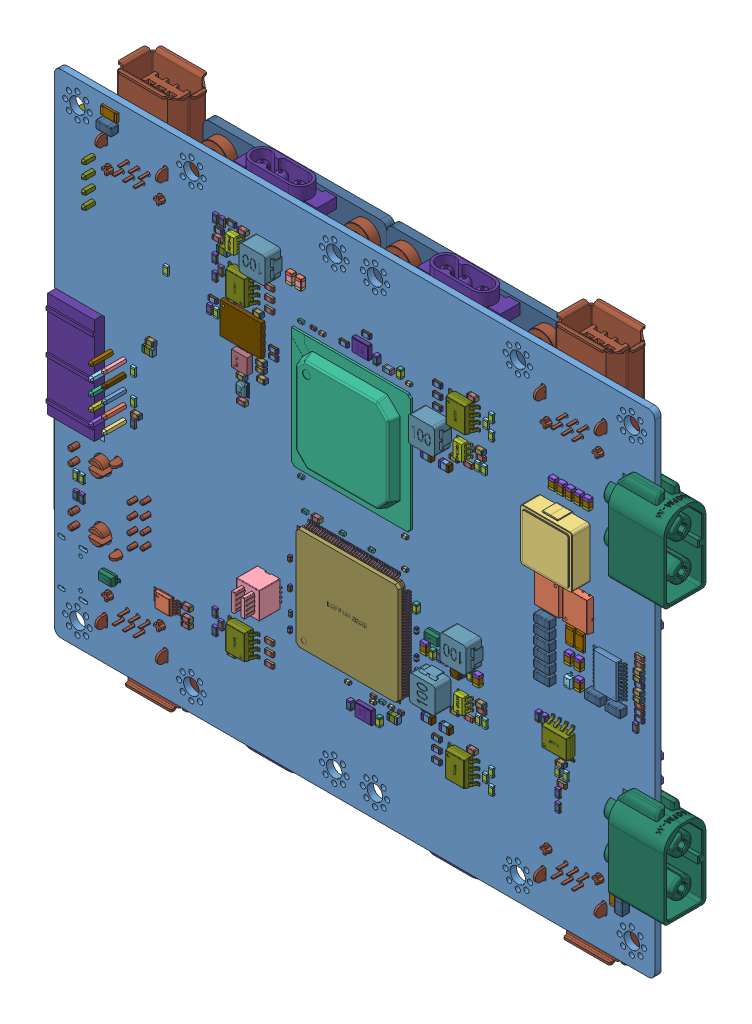
SolidWorks assembly Mother  Board, configuration 默认. Lengths in mm. (continued)
Components (placement in the parent): (continued)
- Mother  Board.step-1: Mother  Board.step [默认] at origin size (122.6 102.08 21) (continued)
  - C120.step-1: C120.step [默认] at origin size (0.8 1.6 0.8) (continued)
    - 5993853744.step-1: 5993853744.step [默认] at (62.7379 73.0251 0) x (0 1 0) z (0 0 1) size (1.6 0.8 0.8) (continued)
      - Terminal-15.step-1: Terminal-15.step [默认] at (-0.8 -0.4 0) size (1.6 0.8 0.8)
        - Open_CASCADE_STEP_translator_6.8_47.1.1-54.step-1: Open_CASCADE_STEP_translator_6.8_47.1.1-54.step [默认] at origin size (0.3 0.8 0.8)
        - Open_CASCADE_STEP_translator_6.8_47.1.2-55.step-1: Open_CASCADE_STEP_translator_6.8_47.1.2-55.step [默认] at origin size (0.3 0.8 0.8)
      - Mid_Body-6.step-1: Mid_Body-6.step [默认] at (-0.8 -0.4 0) size (1 0.8 0.8)
        - Open_CASCADE_STEP_translator_6.8_47.2.1-56.step-1: Open_CASCADE_STEP_translator_6.8_47.2.1-56.step [默认] at origin size (1 0.8 0.8)
  - C119.step-1: C119.step [默认] at origin size (1 0.5 0.5)
    - 5993845664.step-1: 5993845664.step [默认] at (58.9671 58.9279 -1.2164) x (1 0 0) z (0 0 -1) size (1 0.5 0.5)
      - Terminal-2.step-1: Terminal-2.step [默认] at (-0.5 -0.25 0) size (1 0.5 0.5)
        - Open_CASCADE_STEP_translator_6.8_54.1.1.step-1: Open_CASCADE_STEP_translator_6.8_54.1.1.step [默认] at origin size (0.25 0.5 0.5)
        - Open_CASCADE_STEP_translator_6.8_54.1.2.step-1: Open_CASCADE_STEP_translator_6.8_54.1.2.step [默认] at origin size (0.25 0.5 0.5)
      - Mid_Body-1.step-1: Mid_Body-1.step [默认] at (-0.5 -0.25 0) size (0.5 0.5 0.5)
        - Open_CASCADE_STEP_translator_6.8_54.2.1.step-1: Open_CASCADE_STEP_translator_6.8_54.2.1.step [默认] at origin size (0.5 0.5 0.5)
  - C118.step-1: C118.step [默认] at origin size (0.5 1 0.5)
    - 5993845904.step-1: 5993845904.step [默认] at (53.4671 60.4281 -1.2164) x (0 1 0) z (0 0 -1) size (1 0.5 0.5)
      - Terminal-18.step-1: Terminal-18.step [默认] at (-0.5 -0.25 0) size (1 0.5 0.5)
        - Open_CASCADE_STEP_translator_6.8_54.1.1-66.step-1: Open_CASCADE_STEP_translator_6.8_54.1.1-66.step [默认] at origin size (0.25 0.5 0.5)
        - Open_CASCADE_STEP_translator_6.8_54.1.2-67.step-1: Open_CASCADE_STEP_translator_6.8_54.1.2-67.step [默认] at origin size (0.25 0.5 0.5)
      - Mid_Body-9.step-1: Mid_Body-9.step [默认] at (-0.5 -0.25 0) size (0.5 0.5 0.5)
        - Open_CASCADE_STEP_translator_6.8_54.2.1-68.step-1: Open_CASCADE_STEP_translator_6.8_54.2.1-68.step [默认] at origin size (0.5 0.5 0.5)
  - C117.step-1: C117.step [默认] at origin size (0.5 1 0.5)
    - 5993845904.step-1: 5993845904.step [默认] at (53.4671 64.4281 -1.2164) x (0 1 0) z (0 0 -1) size (1 0.5 0.5)
      - Terminal-18.step-1: Terminal-18.step [默认] at (-0.5 -0.25 0) size (1 0.5 0.5)
        - Open_CASCADE_STEP_translator_6.8_54.1.1-66.step-1: Open_CASCADE_STEP_translator_6.8_54.1.1-66.step [默认] at origin size (0.25 0.5 0.5)
        - Open_CASCADE_STEP_translator_6.8_54.1.2-67.step-1: Open_CASCADE_STEP_translator_6.8_54.1.2-67.step [默认] at origin size (0.25 0.5 0.5)
      - Mid_Body-9.step-1: Mid_Body-9.step [默认] at (-0.5 -0.25 0) size (0.5 0.5 0.5)
        - Open_CASCADE_STEP_translator_6.8_54.2.1-68.step-1: Open_CASCADE_STEP_translator_6.8_54.2.1-68.step [默认] at origin size (0.5 0.5 0.5)
  - C115.step-1: C115.step [默认] at origin size (0.5 1 0.5)
    - 5993846064.step-1: 5993846064.step [默认] at (53.4669 62.4279 -1.2164) x (0 -1 0) z (0 0 -1) size (1 0.5 0.5)
      - Terminal-5.step-1: Terminal-5.step [默认] at (-0.5 -0.25 0) size (1 0.5 0.5)
        - Open_CASCADE_STEP_translator_6.8_54.1.1-7.step-1: Open_CASCADE_STEP_translator_6.8_54.1.1-7.step [默认] at origin size (0.25 0.5 0.5)
        - Open_CASCADE_STEP_translator_6.8_54.1.2-8.step-1: Open_CASCADE_STEP_translator_6.8_54.1.2-8.step [默认] at origin size (0.25 0.5 0.5)
      - Mid_Body-4.step-1: Mid_Body-4.step [默认] at (-0.5 -0.25 0) size (0.5 0.5 0.5)
        - Open_CASCADE_STEP_translator_6.8_54.2.1-9.step-1: Open_CASCADE_STEP_translator_6.8_54.2.1-9.step [默认] at origin size (0.5 0.5 0.5)
  - C114.step-1: C114.step [默认] at origin size (0.5 1 0.5)
    - 5993846064.step-1: 5993846064.step [默认] at (53.4669 57.4279 -1.2164) x (0 -1 0) z (0 0 -1) size (1 0.5 0.5)
      - Terminal-5.step-1: Terminal-5.step [默认] at (-0.5 -0.25 0) size (1 0.5 0.5)
        - Open_CASCADE_STEP_translator_6.8_54.1.1-7.step-1: Open_CASCADE_STEP_translator_6.8_54.1.1-7.step [默认] at origin size (0.25 0.5 0.5)
        - Open_CASCADE_STEP_translator_6.8_54.1.2-8.step-1: Open_CASCADE_STEP_translator_6.8_54.1.2-8.step [默认] at origin size (0.25 0.5 0.5)
      - Mid_Body-4.step-1: Mid_Body-4.step [默认] at (-0.5 -0.25 0) size (0.5 0.5 0.5)
        - Open_CASCADE_STEP_translator_6.8_54.2.1-9.step-1: Open_CASCADE_STEP_translator_6.8_54.2.1-9.step [默认] at origin size (0.5 0.5 0.5)
  - C113.step-1: C113.step [默认] at origin size (1 0.5 0.5)
    - 5993845664.step-1: 5993845664.step [默认] at (54.9671 58.9279 -1.2164) x (1 0 0) z (0 0 -1) size (1 0.5 0.5)
      - Terminal-2.step-1: Terminal-2.step [默认] at (-0.5 -0.25 0) size (1 0.5 0.5)
        - Open_CASCADE_STEP_translator_6.8_54.1.1.step-1: Open_CASCADE_STEP_translator_6.8_54.1.1.step [默认] at origin size (0.25 0.5 0.5)
        - Open_CASCADE_STEP_translator_6.8_54.1.2.step-1: Open_CASCADE_STEP_translator_6.8_54.1.2.step [默认] at origin size (0.25 0.5 0.5)
      - Mid_Body-1.step-1: Mid_Body-1.step [默认] at (-0.5 -0.25 0) size (0.5 0.5 0.5)
        - Open_CASCADE_STEP_translator_6.8_54.2.1.step-1: Open_CASCADE_STEP_translator_6.8_54.2.1.step [默认] at origin size (0.5 0.5 0.5)
  - C112.step-1: C112.step [默认] at origin size (1 0.5 0.5)
    - 5993845104.step-1: 5993845104.step [默认] at (56.9669 58.9281 -1.2164) x (-1 0 0) z (0 0 -1) size (1 0.5 0.5)
      - Terminal-3.step-1: Terminal-3.step [默认] at (-0.5 -0.25 0) size (1 0.5 0.5)
        - Open_CASCADE_STEP_translator_6.8_54.1.1-1.step-1: Open_CASCADE_STEP_translator_6.8_54.1.1-1.step [默认] at origin size (0.25 0.5 0.5)
        - Open_CASCADE_STEP_translator_6.8_54.1.2-2.step-1: Open_CASCADE_STEP_translator_6.8_54.1.2-2.step [默认] at origin size (0.25 0.5 0.5)
      - Mid_Body-2.step-1: Mid_Body-2.step [默认] at (-0.5 -0.25 0) size (0.5 0.5 0.5)
        - Open_CASCADE_STEP_translator_6.8_54.2.1-3.step-1: Open_CASCADE_STEP_translator_6.8_54.2.1-3.step [默认] at origin size (0.5 0.5 0.5)
  - C111.step-1: C111.step [默认] at origin size (1 0.5 0.5)
    - 5993845104.step-1: 5993845104.step [默认] at (48.9669 52.9201 -1.2164) x (-1 0 0) z (0 0 -1) size (1 0.5 0.5)
      - Terminal-3.step-1: Terminal-3.step [默认] at (-0.5 -0.25 0) size (1 0.5 0.5)
        - Open_CASCADE_STEP_translator_6.8_54.1.1-1.step-1: Open_CASCADE_STEP_translator_6.8_54.1.1-1.step [默认] at origin size (0.25 0.5 0.5)
        - Open_CASCADE_STEP_translator_6.8_54.1.2-2.step-1: Open_CASCADE_STEP_translator_6.8_54.1.2-2.step [默认] at origin size (0.25 0.5 0.5)
      - Mid_Body-2.step-1: Mid_Body-2.step [默认] at (-0.5 -0.25 0) size (0.5 0.5 0.5)
        - Open_CASCADE_STEP_translator_6.8_54.2.1-3.step-1: Open_CASCADE_STEP_translator_6.8_54.2.1-3.step [默认] at origin size (0.5 0.5 0.5)
  - C110.step-1: C110.step [默认] at origin size (1 0.5 0.5)
    - 5993845104.step-1: 5993845104.step [默认] at (47.9669 58.9281 -1.2164) x (-1 0 0) z (0 0 -1) size (1 0.5 0.5)
      - Terminal-3.step-1: Terminal-3.step [默认] at (-0.5 -0.25 0) size (1 0.5 0.5)
        - Open_CASCADE_STEP_translator_6.8_54.1.1-1.step-1: Open_CASCADE_STEP_translator_6.8_54.1.1-1.step [默认] at origin size (0.25 0.5 0.5)
        - Open_CASCADE_STEP_translator_6.8_54.1.2-2.step-1: Open_CASCADE_STEP_translator_6.8_54.1.2-2.step [默认] at origin size (0.25 0.5 0.5)
      - Mid_Body-2.step-1: Mid_Body-2.step [默认] at (-0.5 -0.25 0) size (0.5 0.5 0.5)
        - Open_CASCADE_STEP_translator_6.8_54.2.1-3.step-1: Open_CASCADE_STEP_translator_6.8_54.2.1-3.step [默认] at origin size (0.5 0.5 0.5)
  - C109.step-1: C109.step [默认] at origin size (1 0.5 0.5)
    - 5993845104.step-1: 5993845104.step [默认] at (51.9669 58.9281 -1.2164) x (-1 0 0) z (0 0 -1) size (1 0.5 0.5)
      - Terminal-3.step-1: Terminal-3.step [默认] at (-0.5 -0.25 0) size (1 0.5 0.5)
        - Open_CASCADE_STEP_translator_6.8_54.1.1-1.step-1: Open_CASCADE_STEP_translator_6.8_54.1.1-1.step [默认] at origin size (0.25 0.5 0.5)
        - Open_CASCADE_STEP_translator_6.8_54.1.2-2.step-1: Open_CASCADE_STEP_translator_6.8_54.1.2-2.step [默认] at origin size (0.25 0.5 0.5)
      - Mid_Body-2.step-1: Mid_Body-2.step [默认] at (-0.5 -0.25 0) size (0.5 0.5 0.5)
        - Open_CASCADE_STEP_translator_6.8_54.2.1-3.step-1: Open_CASCADE_STEP_translator_6.8_54.2.1-3.step [默认] at origin size (0.5 0.5 0.5)
  - C108.step-1: C108.step [默认] at origin size (0.5 1 0.5)
    - 5993846064.step-1: 5993846064.step [默认] at (53.4669 53.4279 -1.2164) x (0 -1 0) z (0 0 -1) size (1 0.5 0.5)
      - Terminal-5.step-1: Terminal-5.step [默认] at (-0.5 -0.25 0) size (1 0.5 0.5)
        - Open_CASCADE_STEP_translator_6.8_54.1.1-7.step-1: Open_CASCADE_STEP_translator_6.8_54.1.1-7.step [默认] at origin size (0.25 0.5 0.5)
        - Open_CASCADE_STEP_translator_6.8_54.1.2-8.step-1: Open_CASCADE_STEP_translator_6.8_54.1.2-8.step [默认] at origin size (0.25 0.5 0.5)
      - Mid_Body-4.step-1: Mid_Body-4.step [默认] at (-0.5 -0.25 0) size (0.5 0.5 0.5)
        - Open_CASCADE_STEP_translator_6.8_54.2.1-9.step-1: Open_CASCADE_STEP_translator_6.8_54.2.1-9.step [默认] at origin size (0.5 0.5 0.5)
  - C107.step-1: C107.step [默认] at origin size (1 0.5 0.5)
    - 5993845664.step-1: 5993845664.step [默认] at (49.9671 58.9279 -1.2164) x (1 0 0) z (0 0 -1) size (1 0.5 0.5)
      - Terminal-2.step-1: Terminal-2.step [默认] at (-0.5 -0.25 0) size (1 0.5 0.5)
        - Open_CASCADE_STEP_translator_6.8_54.1.1.step-1: Open_CASCADE_STEP_translator_6.8_54.1.1.step [默认] at origin size (0.25 0.5 0.5)
        - Open_CASCADE_STEP_translator_6.8_54.1.2.step-1: Open_CASCADE_STEP_translator_6.8_54.1.2.step [默认] at origin size (0.25 0.5 0.5)
      - Mid_Body-1.step-1: Mid_Body-1.step [默认] at (-0.5 -0.25 0) size (0.5 0.5 0.5)
        - Open_CASCADE_STEP_translator_6.8_54.2.1.step-1: Open_CASCADE_STEP_translator_6.8_54.2.1.step [默认] at origin size (0.5 0.5 0.5)
  - C106.step-1: C106.step [默认] at origin size (0.5 1 0.5)
    - 5993845904.step-1: 5993845904.step [默认] at (53.4671 55.4281 -1.2164) x (0 1 0) z (0 0 -1) size (1 0.5 0.5)
      - Terminal-18.step-1: Terminal-18.step [默认] at (-0.5 -0.25 0) size (1 0.5 0.5)
        - Open_CASCADE_STEP_translator_6.8_54.1.1-66.step-1: Open_CASCADE_STEP_translator_6.8_54.1.1-66.step [默认] at origin size (0.25 0.5 0.5)
        - Open_CASCADE_STEP_translator_6.8_54.1.2-67.step-1: Open_CASCADE_STEP_translator_6.8_54.1.2-67.step [默认] at origin size (0.25 0.5 0.5)
      - Mid_Body-9.step-1: Mid_Body-9.step [默认] at (-0.5 -0.25 0) size (0.5 0.5 0.5)
        - Open_CASCADE_STEP_translator_6.8_54.2.1-68.step-1: Open_CASCADE_STEP_translator_6.8_54.2.1-68.step [默认] at origin size (0.5 0.5 0.5)
  - C105.step-1: C105.step [默认] at origin size (1 0.5 0.5)
    - 5993845104.step-1: 5993845104.step [默认] at (50.9669 52.9201 -1.2164) x (-1 0 0) z (0 0 -1) size (1 0.5 0.5)
      - Terminal-3.step-1: Terminal-3.step [默认] at (-0.5 -0.25 0) size (1 0.5 0.5)
        - Open_CASCADE_STEP_translator_6.8_54.1.1-1.step-1: Open_CASCADE_STEP_translator_6.8_54.1.1-1.step [默认] at origin size (0.25 0.5 0.5)
        - Open_CASCADE_STEP_translator_6.8_54.1.2-2.step-1: Open_CASCADE_STEP_translator_6.8_54.1.2-2.step [默认] at origin size (0.25 0.5 0.5)
      - Mid_Body-2.step-1: Mid_Body-2.step [默认] at (-0.5 -0.25 0) size (0.5 0.5 0.5)
        - Open_CASCADE_STEP_translator_6.8_54.2.1-3.step-1: Open_CASCADE_STEP_translator_6.8_54.2.1-3.step [默认] at origin size (0.5 0.5 0.5)
  - C104.step-1: C104.step [默认] at origin size (0.5 1 0.5)
    - 5993845904.step-1: 5993845904.step [默认] at (47.4591 55.4281 -1.2164) x (0 1 0) z (0 0 -1) size (1 0.5 0.5)
      - Terminal-18.step-1: Terminal-18.step [默认] at (-0.5 -0.25 0) size (1 0.5 0.5)
        - Open_CASCADE_STEP_translator_6.8_54.1.1-66.step-1: Open_CASCADE_STEP_translator_6.8_54.1.1-66.step [默认] at origin size (0.25 0.5 0.5)
        - Open_CASCADE_STEP_translator_6.8_54.1.2-67.step-1: Open_CASCADE_STEP_translator_6.8_54.1.2-67.step [默认] at origin size (0.25 0.5 0.5)
      - Mid_Body-9.step-1: Mid_Body-9.step [默认] at (-0.5 -0.25 0) size (0.5 0.5 0.5)
        - Open_CASCADE_STEP_translator_6.8_54.2.1-68.step-1: Open_CASCADE_STEP_translator_6.8_54.2.1-68.step [默认] at origin size (0.5 0.5 0.5)
  - C103.step-1: C103.step [默认] at origin size (1.6 0.8 0.8)
    - 5993853264.step-1: 5993853264.step [默认] at (35.2959 69.2149 0) x (-1 0 0) z (0 0 1) size (1.6 0.8 0.8)
      - Terminal-6.step-1: Terminal-6.step [默认] at (-0.8 -0.4 0) size (1.6 0.8 0.8)
        - Open_CASCADE_STEP_translator_6.8_47.1.1-10.step-1: Open_CASCADE_STEP_translator_6.8_47.1.1-10.step [默认] at origin size (0.3 0.8 0.8)
        - Open_CASCADE_STEP_translator_6.8_47.1.2-11.step-1: Open_CASCADE_STEP_translator_6.8_47.1.2-11.step [默认] at origin size (0.3 0.8 0.8)
      - Mid_Body-5.step-1: Mid_Body-5.step [默认] at (-0.8 -0.4 0) size (1 0.8 0.8)
        - Open_CASCADE_STEP_translator_6.8_47.2.1-12.step-1: Open_CASCADE_STEP_translator_6.8_47.2.1-12.step [默认] at origin size (1 0.8 0.8)
  - C102.step-1: C102.step [默认] at origin size (1 0.5 0.5)
    - 5993845104.step-1: 5993845104.step [默认] at (48.9669 64.9361 -1.2164) x (-1 0 0) z (0 0 -1) size (1 0.5 0.5)
      - Terminal-3.step-1: Terminal-3.step [默认] at (-0.5 -0.25 0) size (1 0.5 0.5)
        - Open_CASCADE_STEP_translator_6.8_54.1.1-1.step-1: Open_CASCADE_STEP_translator_6.8_54.1.1-1.step [默认] at origin size (0.25 0.5 0.5)
        - Open_CASCADE_STEP_translator_6.8_54.1.2-2.step-1: Open_CASCADE_STEP_translator_6.8_54.1.2-2.step [默认] at origin size (0.25 0.5 0.5)
      - Mid_Body-2.step-1: Mid_Body-2.step [默认] at (-0.5 -0.25 0) size (0.5 0.5 0.5)
        - Open_CASCADE_STEP_translator_6.8_54.2.1-3.step-1: Open_CASCADE_STEP_translator_6.8_54.2.1-3.step [默认] at origin size (0.5 0.5 0.5)
  - C101.step-1: C101.step [默认] at origin size (0.5 1 0.5)
    - 5993845904.step-1: 5993845904.step [默认] at (59.4751 55.4281 -1.2164) x (0 1 0) z (0 0 -1) size (1 0.5 0.5)
      - Terminal-18.step-1: Terminal-18.step [默认] at (-0.5 -0.25 0) size (1 0.5 0.5)
        - Open_CASCADE_STEP_translator_6.8_54.1.1-66.step-1: Open_CASCADE_STEP_translator_6.8_54.1.1-66.step [默认] at origin size (0.25 0.5 0.5)
        - Open_CASCADE_STEP_translator_6.8_54.1.2-67.step-1: Open_CASCADE_STEP_translator_6.8_54.1.2-67.step [默认] at origin size (0.25 0.5 0.5)
      - Mid_Body-9.step-1: Mid_Body-9.step [默认] at (-0.5 -0.25 0) size (0.5 0.5 0.5)
        - Open_CASCADE_STEP_translator_6.8_54.2.1-68.step-1: Open_CASCADE_STEP_translator_6.8_54.2.1-68.step [默认] at origin size (0.5 0.5 0.5)
  - C99.step-1: C99.step [默认] at origin size (0.5 1 0.5)
    - 5993845904.step-1: 5993845904.step [默认] at (47.4591 64.4281 -1.2164) x (0 1 0) z (0 0 -1) size (1 0.5 0.5)
      - Terminal-18.step-1: Terminal-18.step [默认] at (-0.5 -0.25 0) size (1 0.5 0.5)
        - Open_CASCADE_STEP_translator_6.8_54.1.1-66.step-1: Open_CASCADE_STEP_translator_6.8_54.1.1-66.step [默认] at origin size (0.25 0.5 0.5)
        - Open_CASCADE_STEP_translator_6.8_54.1.2-67.step-1: Open_CASCADE_STEP_translator_6.8_54.1.2-67.step [默认] at origin size (0.25 0.5 0.5)
      - Mid_Body-9.step-1: Mid_Body-9.step [默认] at (-0.5 -0.25 0) size (0.5 0.5 0.5)
        - Open_CASCADE_STEP_translator_6.8_54.2.1-68.step-1: Open_CASCADE_STEP_translator_6.8_54.2.1-68.step [默认] at origin size (0.5 0.5 0.5)
  - C98.step-1: C98.step [默认] at origin size (0.5 1 0.5)
    - 5993845904.step-1: 5993845904.step [默认] at (59.4751 64.4281 -1.2164) x (0 1 0) z (0 0 -1) size (1 0.5 0.5)
      - Terminal-18.step-1: Terminal-18.step [默认] at (-0.5 -0.25 0) size (1 0.5 0.5)
        - Open_CASCADE_STEP_translator_6.8_54.1.1-66.step-1: Open_CASCADE_STEP_translator_6.8_54.1.1-66.step [默认] at origin size (0.25 0.5 0.5)
        - Open_CASCADE_STEP_translator_6.8_54.1.2-67.step-1: Open_CASCADE_STEP_translator_6.8_54.1.2-67.step [默认] at origin size (0.25 0.5 0.5)
      - Mid_Body-9.step-1: Mid_Body-9.step [默认] at (-0.5 -0.25 0) size (0.5 0.5 0.5)
        - Open_CASCADE_STEP_translator_6.8_54.2.1-68.step-1: Open_CASCADE_STEP_translator_6.8_54.2.1-68.step [默认] at origin size (0.5 0.5 0.5)
  - C97.step-1: C97.step [默认] at origin size (0.5 1 0.5)
    - 5993846064.step-1: 5993846064.step [默认] at (59.4749 60.4279 -1.2164) x (0 -1 0) z (0 0 -1) size (1 0.5 0.5)
      - Terminal-5.step-1: Terminal-5.step [默认] at (-0.5 -0.25 0) size (1 0.5 0.5)
        - Open_CASCADE_STEP_translator_6.8_54.1.1-7.step-1: Open_CASCADE_STEP_translator_6.8_54.1.1-7.step [默认] at origin size (0.25 0.5 0.5)
        - Open_CASCADE_STEP_translator_6.8_54.1.2-8.step-1: Open_CASCADE_STEP_translator_6.8_54.1.2-8.step [默认] at origin size (0.25 0.5 0.5)
      - Mid_Body-4.step-1: Mid_Body-4.step [默认] at (-0.5 -0.25 0) size (0.5 0.5 0.5)
        - Open_CASCADE_STEP_translator_6.8_54.2.1-9.step-1: Open_CASCADE_STEP_translator_6.8_54.2.1-9.step [默认] at origin size (0.5 0.5 0.5)
  - C96.step-1: C96.step [默认] at origin size (0.5 1 0.5)
    - 5993846064.step-1: 5993846064.step [默认] at (59.4749 57.4279 -1.2164) x (0 -1 0) z (0 0 -1) size (1 0.5 0.5)
      - Terminal-5.step-1: Terminal-5.step [默认] at (-0.5 -0.25 0) size (1 0.5 0.5)
        - Open_CASCADE_STEP_translator_6.8_54.1.1-7.step-1: Open_CASCADE_STEP_translator_6.8_54.1.1-7.step [默认] at origin size (0.25 0.5 0.5)
        - Open_CASCADE_STEP_translator_6.8_54.1.2-8.step-1: Open_CASCADE_STEP_translator_6.8_54.1.2-8.step [默认] at origin size (0.25 0.5 0.5)
      - Mid_Body-4.step-1: Mid_Body-4.step [默认] at (-0.5 -0.25 0) size (0.5 0.5 0.5)
        - Open_CASCADE_STEP_translator_6.8_54.2.1-9.step-1: Open_CASCADE_STEP_translator_6.8_54.2.1-9.step [默认] at origin size (0.5 0.5 0.5)
  - C95.step-1: C95.step [默认] at origin size (0.5 1 0.5)
    - 5993846064.step-1: 5993846064.step [默认] at (59.4749 62.4279 -1.2164) x (0 -1 0) z (0 0 -1) size (1 0.5 0.5)
      - Terminal-5.step-1: Terminal-5.step [默认] at (-0.5 -0.25 0) size (1 0.5 0.5)
        - Open_CASCADE_STEP_translator_6.8_54.1.1-7.step-1: Open_CASCADE_STEP_translator_6.8_54.1.1-7.step [默认] at origin size (0.25 0.5 0.5)
        - Open_CASCADE_STEP_translator_6.8_54.1.2-8.step-1: Open_CASCADE_STEP_translator_6.8_54.1.2-8.step [默认] at origin size (0.25 0.5 0.5)
      - Mid_Body-4.step-1: Mid_Body-4.step [默认] at (-0.5 -0.25 0) size (0.5 0.5 0.5)
        - Open_CASCADE_STEP_translator_6.8_54.2.1-9.step-1: Open_CASCADE_STEP_translator_6.8_54.2.1-9.step [默认] at origin size (0.5 0.5 0.5)
  - C94.step-1: C94.step [默认] at origin size (1 0.5 0.5)
    - 5993845104.step-1: 5993845104.step [默认] at (55.9669 52.9201 -1.2164) x (-1 0 0) z (0 0 -1) size (1 0.5 0.5)
      - Terminal-3.step-1: Terminal-3.step [默认] at (-0.5 -0.25 0) size (1 0.5 0.5)
        - Open_CASCADE_STEP_translator_6.8_54.1.1-1.step-1: Open_CASCADE_STEP_translator_6.8_54.1.1-1.step [默认] at origin size (0.25 0.5 0.5)
        - Open_CASCADE_STEP_translator_6.8_54.1.2-2.step-1: Open_CASCADE_STEP_translator_6.8_54.1.2-2.step [默认] at origin size (0.25 0.5 0.5)
      - Mid_Body-2.step-1: Mid_Body-2.step [默认] at (-0.5 -0.25 0) size (0.5 0.5 0.5)
        - Open_CASCADE_STEP_translator_6.8_54.2.1-3.step-1: Open_CASCADE_STEP_translator_6.8_54.2.1-3.step [默认] at origin size (0.5 0.5 0.5)
  - C93.step-1: C93.step [默认] at origin size (1 0.5 0.5)
    - 5993845664.step-1: 5993845664.step [默认] at (57.9671 52.9199 -1.2164) x (1 0 0) z (0 0 -1) size (1 0.5 0.5)
      - Terminal-2.step-1: Terminal-2.step [默认] at (-0.5 -0.25 0) size (1 0.5 0.5)
        - Open_CASCADE_STEP_translator_6.8_54.1.1.step-1: Open_CASCADE_STEP_translator_6.8_54.1.1.step [默认] at origin size (0.25 0.5 0.5)
        - Open_CASCADE_STEP_translator_6.8_54.1.2.step-1: Open_CASCADE_STEP_translator_6.8_54.1.2.step [默认] at origin size (0.25 0.5 0.5)
      - Mid_Body-1.step-1: Mid_Body-1.step [默认] at (-0.5 -0.25 0) size (0.5 0.5 0.5)
        - Open_CASCADE_STEP_translator_6.8_54.2.1.step-1: Open_CASCADE_STEP_translator_6.8_54.2.1.step [默认] at origin size (0.5 0.5 0.5)
  - C92.step-1: C92.step [默认] at origin size (1 0.5 0.5)
    - 5993845664.step-1: 5993845664.step [默认] at (50.9671 64.9359 -1.2164) x (1 0 0) z (0 0 -1) size (1 0.5 0.5)
      - Terminal-2.step-1: Terminal-2.step [默认] at (-0.5 -0.25 0) size (1 0.5 0.5)
        - Open_CASCADE_STEP_translator_6.8_54.1.1.step-1: Open_CASCADE_STEP_translator_6.8_54.1.1.step [默认] at origin size (0.25 0.5 0.5)
        - Open_CASCADE_STEP_translator_6.8_54.1.2.step-1: Open_CASCADE_STEP_translator_6.8_54.1.2.step [默认] at origin size (0.25 0.5 0.5)
      - Mid_Body-1.step-1: Mid_Body-1.step [默认] at (-0.5 -0.25 0) size (0.5 0.5 0.5)
        - Open_CASCADE_STEP_translator_6.8_54.2.1.step-1: Open_CASCADE_STEP_translator_6.8_54.2.1.step [默认] at origin size (0.5 0.5 0.5)
  - C91.step-1: C91.step [默认] at origin size (0.5 1 0.5)
    - 5993846064.step-1: 5993846064.step [默认] at (47.4589 57.4279 -1.2164) x (0 -1 0) z (0 0 -1) size (1 0.5 0.5)
      - Terminal-5.step-1: Terminal-5.step [默认] at (-0.5 -0.25 0) size (1 0.5 0.5)
        - Open_CASCADE_STEP_translator_6.8_54.1.1-7.step-1: Open_CASCADE_STEP_translator_6.8_54.1.1-7.step [默认] at origin size (0.25 0.5 0.5)
        - Open_CASCADE_STEP_translator_6.8_54.1.2-8.step-1: Open_CASCADE_STEP_translator_6.8_54.1.2-8.step [默认] at origin size (0.25 0.5 0.5)
      - Mid_Body-4.step-1: Mid_Body-4.step [默认] at (-0.5 -0.25 0) size (0.5 0.5 0.5)
        - Open_CASCADE_STEP_translator_6.8_54.2.1-9.step-1: Open_CASCADE_STEP_translator_6.8_54.2.1-9.step [默认] at origin size (0.5 0.5 0.5)
  - C89.step-1: C89.step [默认] at origin size (0.5 1 0.5)
    - 5993846064.step-1: 5993846064.step [默认] at (59.4749 53.4279 -1.2164) x (0 -1 0) z (0 0 -1) size (1 0.5 0.5)
      - Terminal-5.step-1: Terminal-5.step [默认] at (-0.5 -0.25 0) size (1 0.5 0.5)
        - Open_CASCADE_STEP_translator_6.8_54.1.1-7.step-1: Open_CASCADE_STEP_translator_6.8_54.1.1-7.step [默认] at origin size (0.25 0.5 0.5)
        - Open_CASCADE_STEP_translator_6.8_54.1.2-8.step-1: Open_CASCADE_STEP_translator_6.8_54.1.2-8.step [默认] at origin size (0.25 0.5 0.5)
      - Mid_Body-4.step-1: Mid_Body-4.step [默认] at (-0.5 -0.25 0) size (0.5 0.5 0.5)
        - Open_CASCADE_STEP_translator_6.8_54.2.1-9.step-1: Open_CASCADE_STEP_translator_6.8_54.2.1-9.step [默认] at origin size (0.5 0.5 0.5)
  - C88.step-1: C88.step [默认] at origin size (1 0.5 0.5)
    - 5993845664.step-1: 5993845664.step [默认] at (57.9671 64.9359 -1.2164) x (1 0 0) z (0 0 -1) size (1 0.5 0.5)
      - Terminal-2.step-1: Terminal-2.step [默认] at (-0.5 -0.25 0) size (1 0.5 0.5)
        - Open_CASCADE_STEP_translator_6.8_54.1.1.step-1: Open_CASCADE_STEP_translator_6.8_54.1.1.step [默认] at origin size (0.25 0.5 0.5)
        - Open_CASCADE_STEP_translator_6.8_54.1.2.step-1: Open_CASCADE_STEP_translator_6.8_54.1.2.step [默认] at origin size (0.25 0.5 0.5)
      - Mid_Body-1.step-1: Mid_Body-1.step [默认] at (-0.5 -0.25 0) size (0.5 0.5 0.5)
        - Open_CASCADE_STEP_translator_6.8_54.2.1.step-1: Open_CASCADE_STEP_translator_6.8_54.2.1.step [默认] at origin size (0.5 0.5 0.5)
  - C87.step-1: C87.step [默认] at origin size (0.5 1 0.5)
    - 5993846064.step-1: 5993846064.step [默认] at (47.4589 62.4279 -1.2164) x (0 -1 0) z (0 0 -1) size (1 0.5 0.5)
      - Terminal-5.step-1: Terminal-5.step [默认] at (-0.5 -0.25 0) size (1 0.5 0.5)
        - Open_CASCADE_STEP_translator_6.8_54.1.1-7.step-1: Open_CASCADE_STEP_translator_6.8_54.1.1-7.step [默认] at origin size (0.25 0.5 0.5)
        - Open_CASCADE_STEP_translator_6.8_54.1.2-8.step-1: Open_CASCADE_STEP_translator_6.8_54.1.2-8.step [默认] at origin size (0.25 0.5 0.5)
      - Mid_Body-4.step-1: Mid_Body-4.step [默认] at (-0.5 -0.25 0) size (0.5 0.5 0.5)
        - Open_CASCADE_STEP_translator_6.8_54.2.1-9.step-1: Open_CASCADE_STEP_translator_6.8_54.2.1-9.step [默认] at origin size (0.5 0.5 0.5)
  - C86.step-1: C86.step [默认] at origin size (1.6 0.8 0.8)
    - 5993853264.step-1: 5993853264.step [默认] at (11.8109 40.5129 0) x (-1 0 0) z (0 0 1) size (1.6 0.8 0.8)
      - Terminal-6.step-1: Terminal-6.step [默认] at (-0.8 -0.4 0) size (1.6 0.8 0.8)
        - Open_CASCADE_STEP_translator_6.8_47.1.1-10.step-1: Open_CASCADE_STEP_translator_6.8_47.1.1-10.step [默认] at origin size (0.3 0.8 0.8)
        - Open_CASCADE_STEP_translator_6.8_47.1.2-11.step-1: Open_CASCADE_STEP_translator_6.8_47.1.2-11.step [默认] at origin size (0.3 0.8 0.8)
      - Mid_Body-5.step-1: Mid_Body-5.step [默认] at (-0.8 -0.4 0) size (1 0.8 0.8)
        - Open_CASCADE_STEP_translator_6.8_47.2.1-12.step-1: Open_CASCADE_STEP_translator_6.8_47.2.1-12.step [默认] at origin size (1 0.8 0.8)
  - C85.step-1: C85.step [默认] at origin size (1 0.5 0.5)
    - 5993845104.step-1: 5993845104.step [默认] at (52.9669 51.9281 -1.2164) x (-1 0 0) z (0 0 -1) size (1 0.5 0.5)
      - Terminal-3.step-1: Terminal-3.step [默认] at (-0.5 -0.25 0) size (1 0.5 0.5)
        - Open_CASCADE_STEP_translator_6.8_54.1.1-1.step-1: Open_CASCADE_STEP_translator_6.8_54.1.1-1.step [默认] at origin size (0.25 0.5 0.5)
        - Open_CASCADE_STEP_translator_6.8_54.1.2-2.step-1: Open_CASCADE_STEP_translator_6.8_54.1.2-2.step [默认] at origin size (0.25 0.5 0.5)
      - Mid_Body-2.step-1: Mid_Body-2.step [默认] at (-0.5 -0.25 0) size (0.5 0.5 0.5)
        - Open_CASCADE_STEP_translator_6.8_54.2.1-3.step-1: Open_CASCADE_STEP_translator_6.8_54.2.1-3.step [默认] at origin size (0.5 0.5 0.5)
  - C84.step-1: C84.step [默认] at origin size (1 0.5 0.5)
    - 5993845104.step-1: 5993845104.step [默认] at (61.9669 64.9361 -1.2164) x (-1 0 0) z (0 0 -1) size (1 0.5 0.5)
      - Terminal-3.step-1: Terminal-3.step [默认] at (-0.5 -0.25 0) size (1 0.5 0.5)
        - Open_CASCADE_STEP_translator_6.8_54.1.1-1.step-1: Open_CASCADE_STEP_translator_6.8_54.1.1-1.step [默认] at origin size (0.25 0.5 0.5)
        - Open_CASCADE_STEP_translator_6.8_54.1.2-2.step-1: Open_CASCADE_STEP_translator_6.8_54.1.2-2.step [默认] at origin size (0.25 0.5 0.5)
      - Mid_Body-2.step-1: Mid_Body-2.step [默认] at (-0.5 -0.25 0) size (0.5 0.5 0.5)
        - Open_CASCADE_STEP_translator_6.8_54.2.1-3.step-1: Open_CASCADE_STEP_translator_6.8_54.2.1-3.step [默认] at origin size (0.5 0.5 0.5)
  - C83.step-1: C83.step [默认] at origin size (1 0.5 0.5)
    - 5993845104.step-1: 5993845104.step [默认] at (50.9669 51.9281 -1.2164) x (-1 0 0) z (0 0 -1) size (1 0.5 0.5)
      - Terminal-3.step-1: Terminal-3.step [默认] at (-0.5 -0.25 0) size (1 0.5 0.5)
        - Open_CASCADE_STEP_translator_6.8_54.1.1-1.step-1: Open_CASCADE_STEP_translator_6.8_54.1.1-1.step [默认] at origin size (0.25 0.5 0.5)
        - Open_CASCADE_STEP_translator_6.8_54.1.2-2.step-1: Open_CASCADE_STEP_translator_6.8_54.1.2-2.step [默认] at origin size (0.25 0.5 0.5)
      - Mid_Body-2.step-1: Mid_Body-2.step [默认] at (-0.5 -0.25 0) size (0.5 0.5 0.5)
        - Open_CASCADE_STEP_translator_6.8_54.2.1-3.step-1: Open_CASCADE_STEP_translator_6.8_54.2.1-3.step [默认] at origin size (0.5 0.5 0.5)
  - C81.step-1: C81.step [默认] at origin size (0.5 1 0.5)
    - 5993845904.step-1: 5993845904.step [默认] at (47.4671 50.4281 -1.2164) x (0 1 0) z (0 0 -1) size (1 0.5 0.5)
      - Terminal-18.step-1: Terminal-18.step [默认] at (-0.5 -0.25 0) size (1 0.5 0.5)
        - Open_CASCADE_STEP_translator_6.8_54.1.1-66.step-1: Open_CASCADE_STEP_translator_6.8_54.1.1-66.step [默认] at origin size (0.25 0.5 0.5)
        - Open_CASCADE_STEP_translator_6.8_54.1.2-67.step-1: Open_CASCADE_STEP_translator_6.8_54.1.2-67.step [默认] at origin size (0.25 0.5 0.5)
      - Mid_Body-9.step-1: Mid_Body-9.step [默认] at (-0.5 -0.25 0) size (0.5 0.5 0.5)
        - Open_CASCADE_STEP_translator_6.8_54.2.1-68.step-1: Open_CASCADE_STEP_translator_6.8_54.2.1-68.step [默认] at origin size (0.5 0.5 0.5)
  - C80.step-1: C80.step [默认] at origin size (1 0.5 0.5)
    - 5993845664.step-1: 5993845664.step [默认] at (59.9671 51.9279 -1.2164) x (1 0 0) z (0 0 -1) size (1 0.5 0.5)
      - Terminal-2.step-1: Terminal-2.step [默认] at (-0.5 -0.25 0) size (1 0.5 0.5)
        - Open_CASCADE_STEP_translator_6.8_54.1.1.step-1: Open_CASCADE_STEP_translator_6.8_54.1.1.step [默认] at origin size (0.25 0.5 0.5)
        - Open_CASCADE_STEP_translator_6.8_54.1.2.step-1: Open_CASCADE_STEP_translator_6.8_54.1.2.step [默认] at origin size (0.25 0.5 0.5)
      - Mid_Body-1.step-1: Mid_Body-1.step [默认] at (-0.5 -0.25 0) size (0.5 0.5 0.5)
        - Open_CASCADE_STEP_translator_6.8_54.2.1.step-1: Open_CASCADE_STEP_translator_6.8_54.2.1.step [默认] at origin size (0.5 0.5 0.5)
  - C79.step-1: C79.step [默认] at origin size (1 0.5 0.5)
    - 5993845104.step-1: 5993845104.step [默认] at (61.9669 62.9361 -1.2164) x (-1 0 0) z (0 0 -1) size (1 0.5 0.5)
      - Terminal-3.step-1: Terminal-3.step [默认] at (-0.5 -0.25 0) size (1 0.5 0.5)
        - Open_CASCADE_STEP_translator_6.8_54.1.1-1.step-1: Open_CASCADE_STEP_translator_6.8_54.1.1-1.step [默认] at origin size (0.25 0.5 0.5)
        - Open_CASCADE_STEP_translator_6.8_54.1.2-2.step-1: Open_CASCADE_STEP_translator_6.8_54.1.2-2.step [默认] at origin size (0.25 0.5 0.5)
      - Mid_Body-2.step-1: Mid_Body-2.step [默认] at (-0.5 -0.25 0) size (0.5 0.5 0.5)
        - Open_CASCADE_STEP_translator_6.8_54.2.1-3.step-1: Open_CASCADE_STEP_translator_6.8_54.2.1-3.step [默认] at origin size (0.5 0.5 0.5)
  - C78.step-1: C78.step [默认] at origin size (1 0.5 0.5)
    - 5993845104.step-1: 5993845104.step [默认] at (61.9669 52.9201 -1.2164) x (-1 0 0) z (0 0 -1) size (1 0.5 0.5)
      - Terminal-3.step-1: Terminal-3.step [默认] at (-0.5 -0.25 0) size (1 0.5 0.5)
        - Open_CASCADE_STEP_translator_6.8_54.1.1-1.step-1: Open_CASCADE_STEP_translator_6.8_54.1.1-1.step [默认] at origin size (0.25 0.5 0.5)
        - Open_CASCADE_STEP_translator_6.8_54.1.2-2.step-1: Open_CASCADE_STEP_translator_6.8_54.1.2-2.step [默认] at origin size (0.25 0.5 0.5)
      - Mid_Body-2.step-1: Mid_Body-2.step [默认] at (-0.5 -0.25 0) size (0.5 0.5 0.5)
        - Open_CASCADE_STEP_translator_6.8_54.2.1-3.step-1: Open_CASCADE_STEP_translator_6.8_54.2.1-3.step [默认] at origin size (0.5 0.5 0.5)
  - C77.step-1: C77.step [默认] at origin size (1 0.5 0.5)
    - 5993845104.step-1: 5993845104.step [默认] at (61.9669 50.9281 -1.2164) x (-1 0 0) z (0 0 -1) size (1 0.5 0.5)
      - Terminal-3.step-1: Terminal-3.step [默认] at (-0.5 -0.25 0) size (1 0.5 0.5)
        - Open_CASCADE_STEP_translator_6.8_54.1.1-1.step-1: Open_CASCADE_STEP_translator_6.8_54.1.1-1.step [默认] at origin size (0.25 0.5 0.5)
        - Open_CASCADE_STEP_translator_6.8_54.1.2-2.step-1: Open_CASCADE_STEP_translator_6.8_54.1.2-2.step [默认] at origin size (0.25 0.5 0.5)
      - Mid_Body-2.step-1: Mid_Body-2.step [默认] at (-0.5 -0.25 0) size (0.5 0.5 0.5)
        - Open_CASCADE_STEP_translator_6.8_54.2.1-3.step-1: Open_CASCADE_STEP_translator_6.8_54.2.1-3.step [默认] at origin size (0.5 0.5 0.5)
  - C76.step-1: C76.step [默认] at origin size (1 0.5 0.5)
    - 5993845104.step-1: 5993845104.step [默认] at (61.9669 58.9281 -1.2164) x (-1 0 0) z (0 0 -1) size (1 0.5 0.5)
      - Terminal-3.step-1: Terminal-3.step [默认] at (-0.5 -0.25 0) size (1 0.5 0.5)
        - Open_CASCADE_STEP_translator_6.8_54.1.1-1.step-1: Open_CASCADE_STEP_translator_6.8_54.1.1-1.step [默认] at origin size (0.25 0.5 0.5)
        - Open_CASCADE_STEP_translator_6.8_54.1.2-2.step-1: Open_CASCADE_STEP_translator_6.8_54.1.2-2.step [默认] at origin size (0.25 0.5 0.5)
      - Mid_Body-2.step-1: Mid_Body-2.step [默认] at (-0.5 -0.25 0) size (0.5 0.5 0.5)
        - Open_CASCADE_STEP_translator_6.8_54.2.1-3.step-1: Open_CASCADE_STEP_translator_6.8_54.2.1-3.step [默认] at origin size (0.5 0.5 0.5)
  - C75.step-1: C75.step [默认] at origin size (0.5 1 0.5)
    - 5993846064.step-1: 5993846064.step [默认] at (53.4669 67.4279 -1.2164) x (0 -1 0) z (0 0 -1) size (1 0.5 0.5)
      - Terminal-5.step-1: Terminal-5.step [默认] at (-0.5 -0.25 0) size (1 0.5 0.5)
        - Open_CASCADE_STEP_translator_6.8_54.1.1-7.step-1: Open_CASCADE_STEP_translator_6.8_54.1.1-7.step [默认] at origin size (0.25 0.5 0.5)
        - Open_CASCADE_STEP_translator_6.8_54.1.2-8.step-1: Open_CASCADE_STEP_translator_6.8_54.1.2-8.step [默认] at origin size (0.25 0.5 0.5)
      - Mid_Body-4.step-1: Mid_Body-4.step [默认] at (-0.5 -0.25 0) size (0.5 0.5 0.5)
        - Open_CASCADE_STEP_translator_6.8_54.2.1-9.step-1: Open_CASCADE_STEP_translator_6.8_54.2.1-9.step [默认] at origin size (0.5 0.5 0.5)
  - C74.step-1: C74.step [默认] at origin size (1 0.5 0.5)
    - 5993845664.step-1: 5993845664.step [默认] at (44.9671 57.9279 -1.2164) x (1 0 0) z (0 0 -1) size (1 0.5 0.5)
      - Terminal-2.step-1: Terminal-2.step [默认] at (-0.5 -0.25 0) size (1 0.5 0.5)
        - Open_CASCADE_STEP_translator_6.8_54.1.1.step-1: Open_CASCADE_STEP_translator_6.8_54.1.1.step [默认] at origin size (0.25 0.5 0.5)
        - Open_CASCADE_STEP_translator_6.8_54.1.2.step-1: Open_CASCADE_STEP_translator_6.8_54.1.2.step [默认] at origin size (0.25 0.5 0.5)
      - Mid_Body-1.step-1: Mid_Body-1.step [默认] at (-0.5 -0.25 0) size (0.5 0.5 0.5)
        - Open_CASCADE_STEP_translator_6.8_54.2.1.step-1: Open_CASCADE_STEP_translator_6.8_54.2.1.step [默认] at origin size (0.5 0.5 0.5)
  - C73.step-1: C73.step [默认] at origin size (0.5 1 0.5)
    - 5993846064.step-1: 5993846064.step [默认] at (57.4589 67.4279 -1.2164) x (0 -1 0) z (0 0 -1) size (1 0.5 0.5)
      - Terminal-5.step-1: Terminal-5.step [默认] at (-0.5 -0.25 0) size (1 0.5 0.5)
        - Open_CASCADE_STEP_translator_6.8_54.1.1-7.step-1: Open_CASCADE_STEP_translator_6.8_54.1.1-7.step [默认] at origin size (0.25 0.5 0.5)
        - Open_CASCADE_STEP_translator_6.8_54.1.2-8.step-1: Open_CASCADE_STEP_translator_6.8_54.1.2-8.step [默认] at origin size (0.25 0.5 0.5)
      - Mid_Body-4.step-1: Mid_Body-4.step [默认] at (-0.5 -0.25 0) size (0.5 0.5 0.5)
        - Open_CASCADE_STEP_translator_6.8_54.2.1-9.step-1: Open_CASCADE_STEP_translator_6.8_54.2.1-9.step [默认] at origin size (0.5 0.5 0.5)
  - C69.step-1: C69.step [默认] at origin size (0.5 1 0.5)
    - 5993846064.step-1: 5993846064.step [默认] at (51.4669 67.4279 -1.2164) x (0 -1 0) z (0 0 -1) size (1 0.5 0.5)
      - Terminal-5.step-1: Terminal-5.step [默认] at (-0.5 -0.25 0) size (1 0.5 0.5)
        - Open_CASCADE_STEP_translator_6.8_54.1.1-7.step-1: Open_CASCADE_STEP_translator_6.8_54.1.1-7.step [默认] at origin size (0.25 0.5 0.5)
        - Open_CASCADE_STEP_translator_6.8_54.1.2-8.step-1: Open_CASCADE_STEP_translator_6.8_54.1.2-8.step [默认] at origin size (0.25 0.5 0.5)
      - Mid_Body-4.step-1: Mid_Body-4.step [默认] at (-0.5 -0.25 0) size (0.5 0.5 0.5)
        - Open_CASCADE_STEP_translator_6.8_54.2.1-9.step-1: Open_CASCADE_STEP_translator_6.8_54.2.1-9.step [默认] at origin size (0.5 0.5 0.5)
  - C68.step-1: C68.step [默认] at origin size (1 0.5 0.5)
    - 5993845664.step-1: 5993845664.step [默认] at (54.9671 51.9279 -1.2164) x (1 0 0) z (0 0 -1) size (1 0.5 0.5)
      - Terminal-2.step-1: Terminal-2.step [默认] at (-0.5 -0.25 0) size (1 0.5 0.5)
        - Open_CASCADE_STEP_translator_6.8_54.1.1.step-1: Open_CASCADE_STEP_translator_6.8_54.1.1.step [默认] at origin size (0.25 0.5 0.5)
        - Open_CASCADE_STEP_translator_6.8_54.1.2.step-1: Open_CASCADE_STEP_translator_6.8_54.1.2.step [默认] at origin size (0.25 0.5 0.5)
      - Mid_Body-1.step-1: Mid_Body-1.step [默认] at (-0.5 -0.25 0) size (0.5 0.5 0.5)
        - Open_CASCADE_STEP_translator_6.8_54.2.1.step-1: Open_CASCADE_STEP_translator_6.8_54.2.1.step [默认] at origin size (0.5 0.5 0.5)
  - C67.step-1: C67.step [默认] at origin size (0.5 1 0.5)
    - 5993846064.step-1: 5993846064.step [默认] at (55.4589 67.4279 -1.2164) x (0 -1 0) z (0 0 -1) size (1 0.5 0.5)
      - Terminal-5.step-1: Terminal-5.step [默认] at (-0.5 -0.25 0) size (1 0.5 0.5)
        - Open_CASCADE_STEP_translator_6.8_54.1.1-7.step-1: Open_CASCADE_STEP_translator_6.8_54.1.1-7.step [默认] at origin size (0.25 0.5 0.5)
        - Open_CASCADE_STEP_translator_6.8_54.1.2-8.step-1: Open_CASCADE_STEP_translator_6.8_54.1.2-8.step [默认] at origin size (0.25 0.5 0.5)
      - Mid_Body-4.step-1: Mid_Body-4.step [默认] at (-0.5 -0.25 0) size (0.5 0.5 0.5)
        - Open_CASCADE_STEP_translator_6.8_54.2.1-9.step-1: Open_CASCADE_STEP_translator_6.8_54.2.1-9.step [默认] at origin size (0.5 0.5 0.5)
  - C66.step-1: C66.step [默认] at origin size (1 0.5 0.5)
    - 5993845664.step-1: 5993845664.step [默认] at (44.9671 61.9199 -1.2164) x (1 0 0) z (0 0 -1) size (1 0.5 0.5)
      - Terminal-2.step-1: Terminal-2.step [默认] at (-0.5 -0.25 0) size (1 0.5 0.5)
        - Open_CASCADE_STEP_translator_6.8_54.1.1.step-1: Open_CASCADE_STEP_translator_6.8_54.1.1.step [默认] at origin size (0.25 0.5 0.5)
        - Open_CASCADE_STEP_translator_6.8_54.1.2.step-1: Open_CASCADE_STEP_translator_6.8_54.1.2.step [默认] at origin size (0.25 0.5 0.5)
      - Mid_Body-1.step-1: Mid_Body-1.step [默认] at (-0.5 -0.25 0) size (0.5 0.5 0.5)
        - Open_CASCADE_STEP_translator_6.8_54.2.1.step-1: Open_CASCADE_STEP_translator_6.8_54.2.1.step [默认] at origin size (0.5 0.5 0.5)
  - C65.step-1: C65.step [默认] at origin size (0.5 1 0.5)
    - 5993846064.step-1: 5993846064.step [默认] at (59.4749 67.4279 -1.2164) x (0 -1 0) z (0 0 -1) size (1 0.5 0.5)
      - Terminal-5.step-1: Terminal-5.step [默认] at (-0.5 -0.25 0) size (1 0.5 0.5)
        - Open_CASCADE_STEP_translator_6.8_54.1.1-7.step-1: Open_CASCADE_STEP_translator_6.8_54.1.1-7.step [默认] at origin size (0.25 0.5 0.5)
        - Open_CASCADE_STEP_translator_6.8_54.1.2-8.step-1: Open_CASCADE_STEP_translator_6.8_54.1.2-8.step [默认] at origin size (0.25 0.5 0.5)
      - Mid_Body-4.step-1: Mid_Body-4.step [默认] at (-0.5 -0.25 0) size (0.5 0.5 0.5)
        - Open_CASCADE_STEP_translator_6.8_54.2.1-9.step-1: Open_CASCADE_STEP_translator_6.8_54.2.1-9.step [默认] at origin size (0.5 0.5 0.5)
  - C63.step-1: C63.step [默认] at origin size (1 0.5 0.5)
    - 5993845664.step-1: 5993845664.step [默认] at (44.9671 63.9279 -1.2164) x (1 0 0) z (0 0 -1) size (1 0.5 0.5)
      - Terminal-2.step-1: Terminal-2.step [默认] at (-0.5 -0.25 0) size (1 0.5 0.5)
        - Open_CASCADE_STEP_translator_6.8_54.1.1.step-1: Open_CASCADE_STEP_translator_6.8_54.1.1.step [默认] at origin size (0.25 0.5 0.5)
        - Open_CASCADE_STEP_translator_6.8_54.1.2.step-1: Open_CASCADE_STEP_translator_6.8_54.1.2.step [默认] at origin size (0.25 0.5 0.5)
      - Mid_Body-1.step-1: Mid_Body-1.step [默认] at (-0.5 -0.25 0) size (0.5 0.5 0.5)
        - Open_CASCADE_STEP_translator_6.8_54.2.1.step-1: Open_CASCADE_STEP_translator_6.8_54.2.1.step [默认] at origin size (0.5 0.5 0.5)
  - C62.step-1: C62.step [默认] at origin size (0.5 1 0.5)
    - 5993846064.step-1: 5993846064.step [默认] at (47.4589 67.4279 -1.2164) x (0 -1 0) z (0 0 -1) size (1 0.5 0.5)
      - Terminal-5.step-1: Terminal-5.step [默认] at (-0.5 -0.25 0) size (1 0.5 0.5)
        - Open_CASCADE_STEP_translator_6.8_54.1.1-7.step-1: Open_CASCADE_STEP_translator_6.8_54.1.1-7.step [默认] at origin size (0.25 0.5 0.5)
        - Open_CASCADE_STEP_translator_6.8_54.1.2-8.step-1: Open_CASCADE_STEP_translator_6.8_54.1.2-8.step [默认] at origin size (0.25 0.5 0.5)
      - Mid_Body-4.step-1: Mid_Body-4.step [默认] at (-0.5 -0.25 0) size (0.5 0.5 0.5)
        - Open_CASCADE_STEP_translator_6.8_54.2.1-9.step-1: Open_CASCADE_STEP_translator_6.8_54.2.1-9.step [默认] at origin size (0.5 0.5 0.5)
  - C61.step-1: C61.step [默认] at origin size (1 0.5 0.5)
    - 5993845664.step-1: 5993845664.step [默认] at (44.9671 51.9279 -1.2164) x (1 0 0) z (0 0 -1) size (1 0.5 0.5)
      - Terminal-2.step-1: Terminal-2.step [默认] at (-0.5 -0.25 0) size (1 0.5 0.5)
        - Open_CASCADE_STEP_translator_6.8_54.1.1.step-1: Open_CASCADE_STEP_translator_6.8_54.1.1.step [默认] at origin size (0.25 0.5 0.5)
        - Open_CASCADE_STEP_translator_6.8_54.1.2.step-1: Open_CASCADE_STEP_translator_6.8_54.1.2.step [默认] at origin size (0.25 0.5 0.5)
      - Mid_Body-1.step-1: Mid_Body-1.step [默认] at (-0.5 -0.25 0) size (0.5 0.5 0.5)
        - Open_CASCADE_STEP_translator_6.8_54.2.1.step-1: Open_CASCADE_STEP_translator_6.8_54.2.1.step [默认] at origin size (0.5 0.5 0.5)
  - C60.step-1: C60.step [默认] at origin size (1 0.5 0.5)
    - 5993845664.step-1: 5993845664.step [默认] at (44.9671 65.9279 -1.2164) x (1 0 0) z (0 0 -1) size (1 0.5 0.5)
      - Terminal-2.step-1: Terminal-2.step [默认] at (-0.5 -0.25 0) size (1 0.5 0.5)
        - Open_CASCADE_STEP_translator_6.8_54.1.1.step-1: Open_CASCADE_STEP_translator_6.8_54.1.1.step [默认] at origin size (0.25 0.5 0.5)
        - Open_CASCADE_STEP_translator_6.8_54.1.2.step-1: Open_CASCADE_STEP_translator_6.8_54.1.2.step [默认] at origin size (0.25 0.5 0.5)
      - Mid_Body-1.step-1: Mid_Body-1.step [默认] at (-0.5 -0.25 0) size (0.5 0.5 0.5)
        - Open_CASCADE_STEP_translator_6.8_54.2.1.step-1: Open_CASCADE_STEP_translator_6.8_54.2.1.step [默认] at origin size (0.5 0.5 0.5)
  - C59.step-1: C59.step [默认] at origin size (1 0.5 0.5)
    - 5993845664.step-1: 5993845664.step [默认] at (44.9671 49.9199 -1.2164) x (1 0 0) z (0 0 -1) size (1 0.5 0.5)
      - Terminal-2.step-1: Terminal-2.step [默认] at (-0.5 -0.25 0) size (1 0.5 0.5)
        - Open_CASCADE_STEP_translator_6.8_54.1.1.step-1: Open_CASCADE_STEP_translator_6.8_54.1.1.step [默认] at origin size (0.25 0.5 0.5)
        - Open_CASCADE_STEP_translator_6.8_54.1.2.step-1: Open_CASCADE_STEP_translator_6.8_54.1.2.step [默认] at origin size (0.25 0.5 0.5)
      - Mid_Body-1.step-1: Mid_Body-1.step [默认] at (-0.5 -0.25 0) size (0.5 0.5 0.5)
        - Open_CASCADE_STEP_translator_6.8_54.2.1.step-1: Open_CASCADE_STEP_translator_6.8_54.2.1.step [默认] at origin size (0.5 0.5 0.5)
  - C58.step-1: C58.step [默认] at origin size (1 0.5 0.5)
    - 5993845104.step-1: 5993845104.step [默认] at (61.9669 57.9361 -1.2164) x (-1 0 0) z (0 0 -1) size (1 0.5 0.5)
      - Terminal-3.step-1: Terminal-3.step [默认] at (-0.5 -0.25 0) size (1 0.5 0.5)
        - Open_CASCADE_STEP_translator_6.8_54.1.1-1.step-1: Open_CASCADE_STEP_translator_6.8_54.1.1-1.step [默认] at origin size (0.25 0.5 0.5)
        - Open_CASCADE_STEP_translator_6.8_54.1.2-2.step-1: Open_CASCADE_STEP_translator_6.8_54.1.2-2.step [默认] at origin size (0.25 0.5 0.5)
      - Mid_Body-2.step-1: Mid_Body-2.step [默认] at (-0.5 -0.25 0) size (0.5 0.5 0.5)
        - Open_CASCADE_STEP_translator_6.8_54.2.1-3.step-1: Open_CASCADE_STEP_translator_6.8_54.2.1-3.step [默认] at origin size (0.5 0.5 0.5)
  - C28.step-1: C28.step [默认] at origin size (1.6 0.8 0.8)
    - 5993853264.step-1: 5993853264.step [默认] at (73.2789 64.1349 0) x (-1 0 0) z (0 0 1) size (1.6 0.8 0.8)
      - Terminal-6.step-1: Terminal-6.step [默认] at (-0.8 -0.4 0) size (1.6 0.8 0.8)
        - Open_CASCADE_STEP_translator_6.8_47.1.1-10.step-1: Open_CASCADE_STEP_translator_6.8_47.1.1-10.step [默认] at origin size (0.3 0.8 0.8)
        - Open_CASCADE_STEP_translator_6.8_47.1.2-11.step-1: Open_CASCADE_STEP_translator_6.8_47.1.2-11.step [默认] at origin size (0.3 0.8 0.8)
      - Mid_Body-5.step-1: Mid_Body-5.step [默认] at (-0.8 -0.4 0) size (1 0.8 0.8)
        - Open_CASCADE_STEP_translator_6.8_47.2.1-12.step-1: Open_CASCADE_STEP_translator_6.8_47.2.1-12.step [默认] at origin size (1 0.8 0.8)
  - C27.step-1: C27.step [默认] at origin size (2.01 1.25 0.94)
    - 5993850784.step-1: 5993850784.step [默认] at (71.5011 61.9761 0) x (1 0 0) z (0 0 1) size (2.01 1.25 0.94)
      - Fillet1.step-1: Fillet1.step [默认] at origin size (0.5 1.25 0.94)
      - Fillet2.step-1: Fillet2.step [默认] at origin size (0.5 1.25 0.94)
      - body2.step-1: body2.step [默认] at origin size (1.01 1.22 0.92)
  - C26.step-1: C26.step [默认] at origin size (1.6 0.8 0.8)
    - 5993854224.step-1: 5993854224.step [默认] at (32.3851 81.5341 0) x (1 0 0) z (0 0 1) size (1.6 0.8 0.8)
